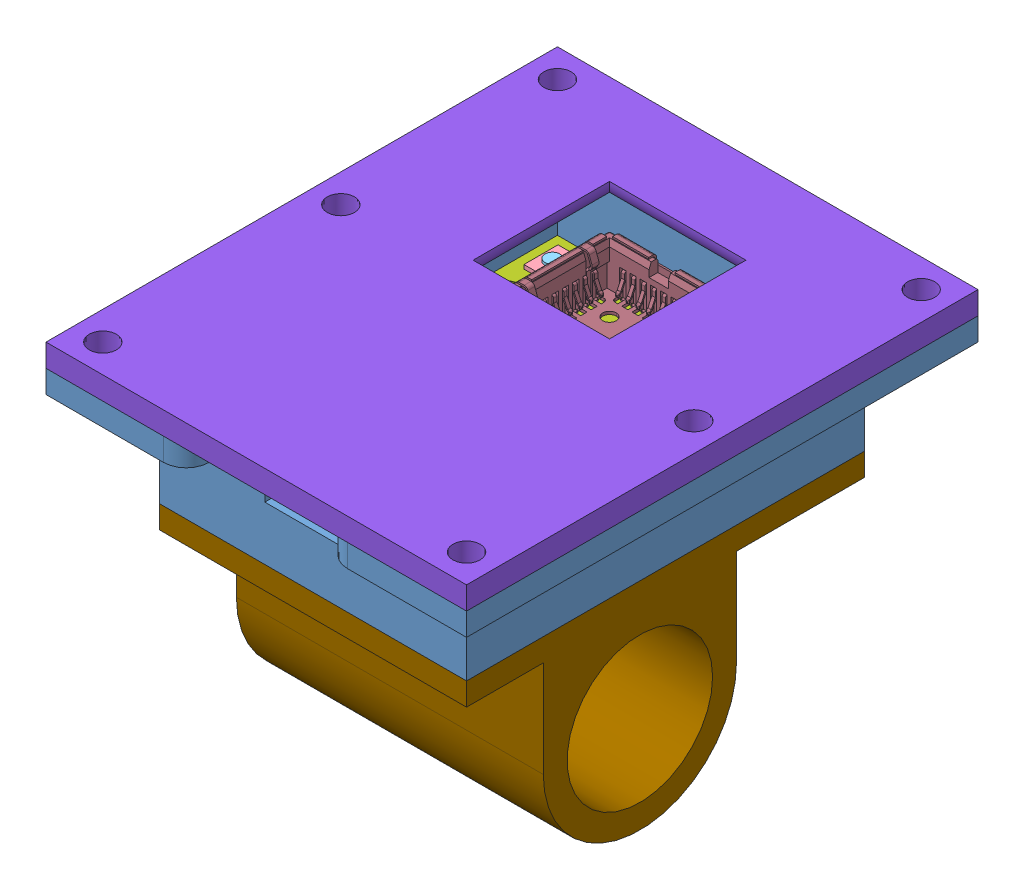
SolidWorks assembly IR Camera Holder, configuration Default. Lengths in mm.
Overall size (37 31.32 45).
184 component instances, 30 part files, 6 mates.
Components (placement in the parent):
- Case_box-1: Case_box [Default] at (12.4279 12.3728 26.2376) size (37 10.32 45)
- PureThermal2.step-1: PureThermal2.step [Default] at (2.416 17.8272 42.1774) x (1 0 0) z (0 1 0) size (22 32.32 9.95)
  - R9.step-1: R9.step [Default] at origin size (1.7 0.8 0.8)
    - 843222320.step-1: 843222320.step [Default] at (7.8994 17.0942 -2.9192) size (1.7 0.8 0.8)
      - Extruded.step-1: Extruded.step [Default] at origin size (1.7 0.8 0.8)
  - R5.step-1: R5.step [Default] at origin size (0.55 1.05 0.55)
    - 443469840.step-1: 443469840.step [Default] at (18.5676 13.4117 0) size (0.55 1.05 0.55)
      - Extruded-0.step-1: Extruded-0.step [Default] at origin size (0.55 1.05 0.55)
  - SW2.step-1: SW2.step [Default] at origin size (3 2 0.58)
    - 859417200.step-1: 859417200.step [Default] at (2.7941 19.8121 0.35) size (1.3 1.3 0.23)
      - Cylinder.step-1: Cylinder.step [Default] at origin size (1.3 1.3 0.23)
    - 443469456.step-1: 443469456.step [Default] at (2.794 19.812 0) size (3 2 0.35)
      - Extruded-1.step-1: Extruded-1.step [Default] at origin size (3 2 0.35)
  - R1.step-1: R1.step [Default] at origin size (1.05 0.55 0.55)
    - 443466128.step-1: 443466128.step [Default] at (11.9711 25.9844 -2.6692) size (1.05 0.55 0.55)
      - Extruded-2.step-1: Extruded-2.step [Default] at origin size (1.05 0.55 0.55)
  - J2.step-1: J2.step [Default] at origin size (2.54 17.78 2.54)
    - 843221040.step-1: 843221040.step [Default] at (20.7264 20.29 0) size (2.54 2.54 2.54)
      - Extruded-3.step-1: Extruded-3.step [Default] at origin size (2.54 2.54 2.54)
    - 843221040.step-2: 843221040.step [Default] at (20.7264 17.75 0) size (2.54 2.54 2.54)
      - Extruded-3.step-1: Extruded-3.step [Default] at origin size (2.54 2.54 2.54)
    - 843221040.step-3: 843221040.step [Default] at (20.7264 15.21 0) size (2.54 2.54 2.54)
      - Extruded-3.step-1: Extruded-3.step [Default] at origin size (2.54 2.54 2.54)
    - 843221040.step-4: 843221040.step [Default] at (20.7264 12.67 0) size (2.54 2.54 2.54)
      - Extruded-3.step-1: Extruded-3.step [Default] at origin size (2.54 2.54 2.54)
    - 843221040.step-5: 843221040.step [Default] at (20.7264 10.13 0) size (2.54 2.54 2.54)
      - Extruded-3.step-1: Extruded-3.step [Default] at origin size (2.54 2.54 2.54)
    - 843221040.step-6: 843221040.step [Default] at (20.7264 7.59 0) size (2.54 2.54 2.54)
      - Extruded-3.step-1: Extruded-3.step [Default] at origin size (2.54 2.54 2.54)
    - 843221040.step-7: 843221040.step [Default] at (20.7264 5.05 0) size (2.54 2.54 2.54)
      - Extruded-3.step-1: Extruded-3.step [Default] at origin size (2.54 2.54 2.54)
  - S2.step-1: S2.step [Default] at origin size (13.66 12.7 0.04)
    - 843220400.step-1: 843220400.step [Default] at (8.03 10.8 2.5019) size (13.66 12.7 0.04)
      - Extruded-4.step-1: Extruded-4.step [Default] at origin size (13.66 12.7 0.04) (hidden)
  - C16.step-1: C16.step [Default] at origin size (1.05 0.55 0.55)
    - 443466128.step-1: 443466128.step [Default] at (13.1323 14.0972 -2.6692) size (1.05 0.55 0.55)
      - Extruded-2.step-1: Extruded-2.step [Default] at origin size (1.05 0.55 0.55)
  - U4.step-1: U4.step [Default] at origin size (3.1 1.8 1.19)
    - 843222064.step-1: 843222064.step [Default] at (12.4714 16.5608 -3.3092) size (3.1 1.8 1.19)
      - Extruded-5.step-1: Extruded-5.step [Default] at origin size (3.1 1.8 1.19)
  - L2.step-1: L2.step [Default] at origin size (2.2 1.45 0.6)
    - 443468688.step-1: 443468688.step [Default] at (7.1628 10.7442 -2.7192) size (2.2 1.45 0.6)
      - Extruded-6.step-1: Extruded-6.step [Default] at origin size (2.2 1.45 0.6)
  - D3.step-1: D3.step [Default] at origin size (0.6 1 0.2)
    - 843221168.step-1: 843221168.step [Default] at (4.45 27.45 0) size (0.6 1 0.2)
      - Extruded-7.step-1: Extruded-7.step [Default] at origin size (0.6 1 0.2)
  - R21.step-1: R21.step [Default] at origin size (0.55 1.05 0.55)
    - 443469840.step-1: 443469840.step [Default] at (4.3998 25.4995 0) size (0.55 1.05 0.55)
      - Extruded-0.step-1: Extruded-0.step [Default] at origin size (0.55 1.05 0.55)
  - C34.step-1: C34.step [Default] at origin size (0.55 1.05 0.55)
    - 443469840.step-1: 443469840.step [Default] at (2.4382 9.4737 0) size (0.55 1.05 0.55)
      - Extruded-0.step-1: Extruded-0.step [Default] at origin size (0.55 1.05 0.55)
  - C15.step-1: C15.step [Default] at origin size (1.05 0.55 0.55)
    - 443466128.step-1: 443466128.step [Default] at (9.2959 6.9344 0) size (1.05 0.55 0.55)
      - Extruded-2.step-1: Extruded-2.step [Default] at origin size (1.05 0.55 0.55)
  - C14.step-1: C14.step [Default] at origin size (0.55 1.05 0.55)
    - 443469840.step-1: 443469840.step [Default] at (11.4806 14.6045 0) size (0.55 1.05 0.55)
      - Extruded-0.step-1: Extruded-0.step [Default] at origin size (0.55 1.05 0.55)
  - C13.step-1: C13.step [Default] at origin size (1.05 0.55 0.55)
    - 443466128.step-1: 443466128.step [Default] at (11.0495 16.1796 0) size (1.05 0.55 0.55)
      - Extruded-2.step-1: Extruded-2.step [Default] at origin size (1.05 0.55 0.55)
  - C12.step-1: C12.step [Default] at origin size (0.55 1.05 0.55)
    - 443469840.step-1: 443469840.step [Default] at (2.3874 6.4257 0) size (0.55 1.05 0.55)
      - Extruded-0.step-1: Extruded-0.step [Default] at origin size (0.55 1.05 0.55)
  - R20.step-1: R20.step [Default] at origin size (1.05 0.55 0.55)
    - 443466128.step-1: 443466128.step [Default] at (19.8115 27.4064 -2.6692) size (1.05 0.55 0.55)
      - Extruded-2.step-1: Extruded-2.step [Default] at origin size (1.05 0.55 0.55)
  - R3.step-1: R3.step [Default] at origin size (1.05 0.55 0.55)
    - 443466128.step-1: 443466128.step [Default] at (19.8115 28.3716 -2.6692) size (1.05 0.55 0.55)
      - Extruded-2.step-1: Extruded-2.step [Default] at origin size (1.05 0.55 0.55)
  - L1.step-1: L1.step [Default] at origin size (2.2 1.45 0.6)
    - 443468688.step-1: 443468688.step [Default] at (11.3538 10.6172 -2.7192) size (2.2 1.45 0.6)
      - Extruded-6.step-1: Extruded-6.step [Default] at origin size (2.2 1.45 0.6)
  - C11.step-1: C11.step [Default] at origin size (1.7 0.8 0.8)
    - 843222320.step-1: 843222320.step [Default] at (19.6342 26.3398 -2.9192) size (1.7 0.8 0.8)
      - Extruded.step-1: Extruded.step [Default] at origin size (1.7 0.8 0.8)
  - C10.step-1: C10.step [Default] at origin size (2.2 1.45 0.6)
    - 443468688.step-1: 443468688.step [Default] at (12.1 12.65 -2.7192) size (2.2 1.45 0.6)
      - Extruded-6.step-1: Extruded-6.step [Default] at origin size (2.2 1.45 0.6)
  - Y1.step-1: Y1.step [Default] at origin size (2.7 3.4 0.95)
    - 843221936.step-1: 843221936.step [Default] at (16.764 18.288 -2.9692) size (2.7 3.4 0.85)
      - Extruded-8.step-1: Extruded-8.step [Default] at origin size (2.7 3.4 0.85)
    - 859416960.step-1: 859416960.step [Default] at (16.239 17.5372 -3.0192) x (0 1 0) z (0 0 -1) size (0.2 0.2 0.05)
      - Cylinder-9.step-1: Cylinder-9.step [Default] at origin size (0.2 0.2 0.05)
  - C8.step-1: C8.step [Default] at origin size (1.05 0.55 0.55)
    - 443466128.step-1: 443466128.step [Default] at (17.2979 15.8244 -2.6692) size (1.05 0.55 0.55)
      - Extruded-2.step-1: Extruded-2.step [Default] at origin size (1.05 0.55 0.55)
  - U1.step-1: U1.step [Default] at origin size (10.78 10.6 4.2)
    - 1050281001.step-1: 1050281001.step [Default] at (11.0501 23.5299 2.1) x (0 -1 0) z (-1 0 0) size (10.6 4.2 10.78)
      - SOLID.step-1: SOLID.step [Default] at origin size (10.6 4.2 10.78)
      - COMPOUND.step-1: COMPOUND.step [Default] at origin
  - C1.step-1: C1.step [Default] at origin size (0.55 1.05 0.55)
    - 443469840.step-1: 443469840.step [Default] at (9.5252 13.2583 -2.6692) size (0.55 1.05 0.55)
      - Extruded-0.step-1: Extruded-0.step [Default] at origin size (0.55 1.05 0.55)
  - C3.step-1: C3.step [Default] at origin size (1.45 2.2 0.6)
    - 443469072.step-1: 443469072.step [Default] at (9.5758 7.9248 -2.7192) size (1.45 2.2 0.6)
      - Extruded-10.step-1: Extruded-10.step [Default] at origin size (1.45 2.2 0.6)
  - C4.step-1: C4.step [Default] at origin size (0.55 1.05 0.55)
    - 443469840.step-1: 443469840.step [Default] at (13.7924 10.5151 -2.6692) size (0.55 1.05 0.55)
      - Extruded-0.step-1: Extruded-0.step [Default] at origin size (0.55 1.05 0.55)
  - C5.step-1: C5.step [Default] at origin size (0.55 1.05 0.55)
    - 443469840.step-1: 443469840.step [Default] at (13.9698 22.4795 -2.6692) size (0.55 1.05 0.55)
      - Extruded-0.step-1: Extruded-0.step [Default] at origin size (0.55 1.05 0.55)
  - C6.step-1: C6.step [Default] at origin size (1.05 0.55 0.55)
    - 443466128.step-1: 443466128.step [Default] at (12.9535 19.2022 -2.6692) size (1.05 0.55 0.55)
      - Extruded-2.step-1: Extruded-2.step [Default] at origin size (1.05 0.55 0.55)
  - C7.step-1: C7.step [Default] at origin size (0.55 1.05 0.55)
    - 443469840.step-1: 443469840.step [Default] at (5.7402 22.5811 -2.6692) size (0.55 1.05 0.55)
      - Extruded-0.step-1: Extruded-0.step [Default] at origin size (0.55 1.05 0.55)
  - U2.step-1: U2.step [Default] at origin size (1.6 2.9 0.8)
    - 843220912.step-1: 843220912.step [Default] at (12.4968 8.1534 -3.0192) size (1.6 2.9 0.8)
      - Extruded-11.step-1: Extruded-11.step [Default] at origin size (1.6 2.9 0.8)
  - C30.step-1: C30.step [Default] at origin size (0.8 1.7 0.8)
    - 443468560.step-1: 443468560.step [Default] at (12.5288 23.5366 -2.9192) size (0.8 1.7 0.8)
      - Extruded-12.step-1: Extruded-12.step [Default] at origin size (0.8 1.7 0.8)
  - C31.step-1: C31.step [Default] at origin size (1.05 0.55 0.55)
    - 443466128.step-1: 443466128.step [Default] at (5.5995 16.8498 -2.6692) size (1.05 0.55 0.55)
      - Extruded-2.step-1: Extruded-2.step [Default] at origin size (1.05 0.55 0.55)
  - R2.step-1: R2.step [Default] at origin size (1.05 0.55 0.55)
    - 443466128.step-1: 443466128.step [Default] at (17.2979 14.91 -2.6692) size (1.05 0.55 0.55)
      - Extruded-2.step-1: Extruded-2.step [Default] at origin size (1.05 0.55 0.55)
  - R19.step-1: R19.step [Default] at origin size (1.05 0.55 0.55)
    - 443466128.step-1: 443466128.step [Default] at (17.2979 13.9956 -2.6692) size (1.05 0.55 0.55)
      - Extruded-2.step-1: Extruded-2.step [Default] at origin size (1.05 0.55 0.55)
  - R6.step-1: R6.step [Default] at origin size (0.55 1.05 0.55)
    - 443469840.step-1: 443469840.step [Default] at (2.4382 11.3279 0) size (0.55 1.05 0.55)
      - Extruded-0.step-1: Extruded-0.step [Default] at origin size (0.55 1.05 0.55)
  - R8.step-1: R8.step [Default] at origin size (1.05 0.55 0.55)
    - 443466128.step-1: 443466128.step [Default] at (17.3741 12.9034 -2.6692) size (1.05 0.55 0.55)
      - Extruded-2.step-1: Extruded-2.step [Default] at origin size (1.05 0.55 0.55)
  - Y2.step-1: Y2.step [Default] at origin size (3.4 2.7 0.95)
    - 843220144.step-1: 843220144.step [Default] at (7.2896 13.5128 -2.9692) size (3.4 2.7 0.85)
      - Extruded-13.step-1: Extruded-13.step [Default] at origin size (3.4 2.7 0.85)
    - 859416720.step-1: 859416720.step [Default] at (8.0404 12.9878 -3.0192) x (-1 0 0) z (0 0 -1) size (0.2 0.2 0.05)
      - Cylinder-14.step-1: Cylinder-14.step [Default] at origin size (0.2 0.2 0.05)
  - U3.step-1: U3.step [Default] at origin size (7 7 0.55)
    - 843221424.step-1: 843221424.step [Default] at (6.985 11.811 0.05) size (7 7 0.55)
      - Extruded-15.step-1: Extruded-15.step [Default] at origin size (7 7 0.55)
  - C9.step-1: C9.step [Default] at origin size (1.45 2.2 0.6)
    - 443469072.step-1: 443469072.step [Default] at (15.113 12.5476 -2.7192) size (1.45 2.2 0.6)
      - Extruded-10.step-1: Extruded-10.step [Default] at origin size (1.45 2.2 0.6)
  - D1.step-1: D1.step [Default] at origin size (1.8 3.75 1)
    - 843222192.step-1: 843222192.step [Default] at (1.27 8.6614 -3.1192) size (1.8 3.75 1)
      - Extruded-16.step-1: Extruded-16.step [Default] at origin size (1.8 3.75 1)
  - C17.step-1: C17.step [Default] at origin size (0.55 1.05 0.55)
    - 443469840.step-1: 443469840.step [Default] at (14.6556 16.5105 -2.6692) size (0.55 1.05 0.55)
      - Extruded-0.step-1: Extruded-0.step [Default] at origin size (0.55 1.05 0.55)
  - C18.step-1: C18.step [Default] at origin size (1.05 0.55 0.55)
    - 443466128.step-1: 443466128.step [Default] at (9.5499 5.7402 -2.6692) size (1.05 0.55 0.55)
      - Extruded-2.step-1: Extruded-2.step [Default] at origin size (1.05 0.55 0.55)
  - C19.step-1: C19.step [Default] at origin size (1.05 0.55 0.55)
    - 443466128.step-1: 443466128.step [Default] at (4.5207 10.617 -2.6692) size (1.05 0.55 0.55)
      - Extruded-2.step-1: Extruded-2.step [Default] at origin size (1.05 0.55 0.55)
  - Rset1.step-1: Rset1.step [Default] at origin size (0.55 1.05 0.55)
    - 443469840.step-1: 443469840.step [Default] at (14.8592 9.8293 -2.6692) size (0.55 1.05 0.55)
      - Extruded-0.step-1: Extruded-0.step [Default] at origin size (0.55 1.05 0.55)
  - Rset2.step-1: Rset2.step [Default] at origin size (0.55 1.05 0.55)
    - 443469840.step-1: 443469840.step [Default] at (14.8592 6.8321 -2.6692) size (0.55 1.05 0.55)
      - Extruded-0.step-1: Extruded-0.step [Default] at origin size (0.55 1.05 0.55)
  - U5.step-1: U5.step [Default] at origin size (3.1 1.8 1)
    - 843220528.step-1: 843220528.step [Default] at (6.985 7.7724 -3.2192) size (3.1 1.8 1)
      - Extruded-17.step-1: Extruded-17.step [Default] at origin size (3.1 1.8 1)
  - S4.step-1: S4.step [Default] at origin size (16.51 16.51 0.03)
    - 909917680.step-1: 909917680.step [Default] at (11 12.79 -5.7514) size (16.51 16.51 0.03)
      - Extruded-18.step-1: Extruded-18.step [Default] at origin size (16.51 16.51 0.03) (hidden)
  - SW1.step-1: SW1.step [Default] at origin size (2 3 0.58)
    - 909917424.step-1: 909917424.step [Default] at (2.1 27.45 0) size (2 3 0.35)
      - Extruded-19.step-1: Extruded-19.step [Default] at origin size (2 3 0.35)
    - 859417080.step-1: 859417080.step [Default] at (2.0999 27.4501 0.35) x (0 1 0) z (0 0 1) size (1.3 1.3 0.23)
      - Cylinder-20.step-1: Cylinder-20.step [Default] at origin size (1.3 1.3 0.23)
  - C20.step-1: C20.step [Default] at origin size (0.55 1.05 0.55)
    - 443469840.step-1: 443469840.step [Default] at (4.9604 14.8597 -2.6692) size (0.55 1.05 0.55)
      - Extruded-0.step-1: Extruded-0.step [Default] at origin size (0.55 1.05 0.55)
  - R4.step-1: R4.step [Default] at origin size (1.05 0.55 0.55)
    - 443466128.step-1: 443466128.step [Default] at (6.2733 6.4264 0) size (1.05 0.55 0.55)
      - Extruded-2.step-1: Extruded-2.step [Default] at origin size (1.05 0.55 0.55)
  - R7.step-1: R7.step [Default] at origin size (1.05 0.55 0.55)
    - 443466128.step-1: 443466128.step [Default] at (10.9987 14.1226 -2.6692) size (1.05 0.55 0.55)
      - Extruded-2.step-1: Extruded-2.step [Default] at origin size (1.05 0.55 0.55)
  - J3.step-1: J3.step [Default] at origin size (8.81 5.63 3.08)
    - COLOR13-1.step-1: COLOR13-1.step [Default] at (11.0491 1.8073 1.39) x (1 0 0) z (0 -1 0) size (8.81 3.08 5.63)
  - Board.step-1: Board.step [Default] at (0 0 -2.1192) size (22 30 2.12)
- Case_lid-1: Case_lid [Default] at (14.4041 24.6928 26.2376) x (-1 0 0) z (0 0 1) size (37 4.4 45)
- Case_thorlabspostmount-1: Case_thorlabspostmount [Default] at (14.4041 12.3728 26.2376) x (-1 0 0) z (0 0 1) size (27 19 35)
Mates (geometry in assembly coordinates):
- Concentric1: concentric anti-aligned: cylinder of Case_box-1 through (4.416 16.3728 40.1774) axis (0 1 0) radius 1.2; cylinder of PureThermal2.step-1/Board.step-1 through (4.416 15.708 40.1774) axis (0 -1 0) radius 1.11
- Coincident1: coincident anti-aligned: plane of Case_box-1 through (4.416 22.6928 40.1774) normal (0 1 0); plane of Case_lid-1 through (14.4041 22.6928 26.2376) normal (0 -1 0)
- Concentric2: concentric anti-aligned: circle of PureThermal2.step-1/Board.step-1; circle of Case_lid-1
- Coincident2: coincident anti-aligned: plane of Case_box-1 through (12.4279 12.3728 26.2376) normal (0 -1 0); plane of Case_thorlabspostmount-1 through (14.4041 12.3728 26.2376) normal (0 1 0)
- Concentric6: concentric anti-aligned: circle of Case_box-1; circle of Case_thorlabspostmount-1
- Concentric7: concentric anti-aligned: cylinder of Case_box-1 through (22.416 16.3728 40.1774) axis (0 1 0) radius 1.2; cylinder of Case_thorlabspostmount-1 through (22.416 10.3728 40.1774) axis (0 -1 0) radius 1.2
